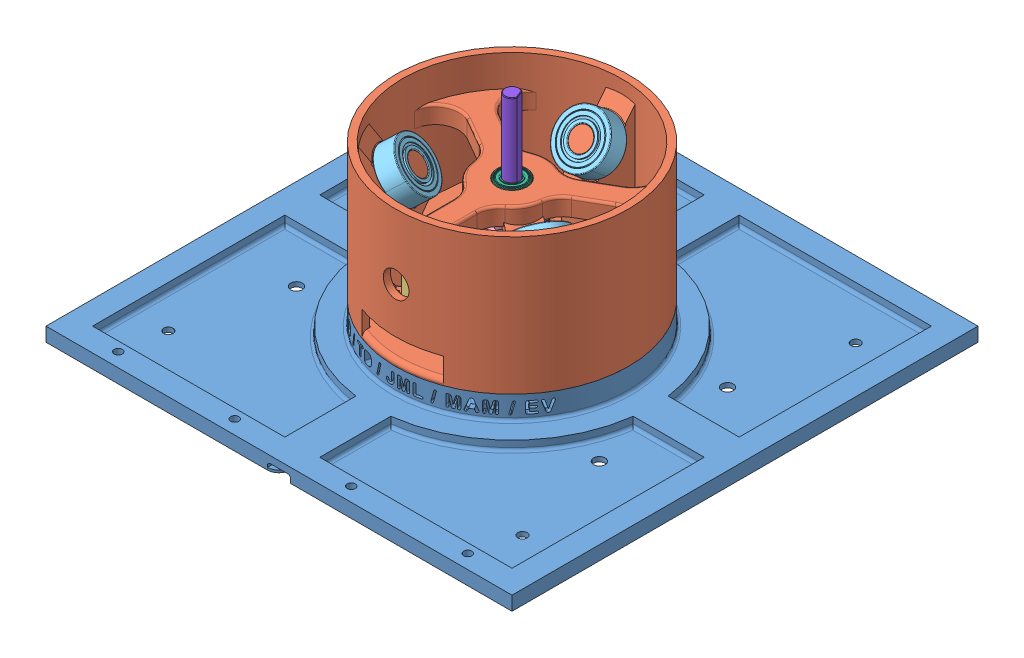
SolidWorks assembly Socle, configuration Défaut. Lengths in mm.
Overall size (200 92.98 200).
27 component instances, 14 part files, 141 mates.
Components (placement in the parent):
- robot_base_plate-2: robot_base_plate [Défaut] at (0 -6 0) size (200 16 200)
- Support_Bearing_V4-1: Support_Bearing_V4 [Défaut] at (0 10 0) x (0 0 1) z (-1 0 0) size (100 58.5 100)
- XL430-W250-1: XL430-W250 [Défaut] at (0 36 0) x (-1 0 0) z (0 1 0) size (28.5 46.5 36.18)
- Coupler_Joint1-1: Coupler_Joint1 [Défaut] at (0 36 0) x (0.374118 0 0.927381) z (-0.927381 0 0.374118) size (22.5 6 20.75)
- bearing-1: bearing [Default] at (0 52.1597 -32.8363) x (0.617014 0.614506 -0.491605) z (0 -0.624695 -0.780869) size (22.23 22.23 8.73)
- bearing-2: bearing [Default] at (-28.437 52.1597 16.4181) x (0.592905 -0.776094 -0.214808) z (-0.676252 -0.624695 0.390434) size (22.23 22.23 8.73)
- bearing-3: bearing [Default] at (28.437 52.1597 16.4181) x (0.541002 0.780869 0.312348) z (0.676252 -0.624695 0.390434) size (22.23 22.23 8.73)
- 535198-1: 535198 [Default] at (0 55.6322 0) x (-0.798975 0 -0.601364) z (-0.601364 0 0.798975) size (13.87 4.75 13.87)
- 6432K12-1: 6432K12 [Défaut] at (0 43.2374 0) x (-0.932842 0 -0.360287) z (0.360287 0 -0.932842) size (12.48 7.15 12.48)
- shaft-1: shaft [2po] at (0 61.5779 0) x (0.374118 0 0.927381) z (0 1 0) size (6.35 5.71 50.8)
- M3-8mm_91292A112_TYPE 18-8 SS SOCKET HEAD CAP SCREW-1: M3-8mm_91292A112_TYPE 18-8 SS SOCKET HEAD CAP SCREW [91292A112] at (2.3555 39 -0.9503) x (0.050445 0.990868 0.125045) z (-0.927381 0 0.374118) size (5.5 5.5 11.2)
- M3-NUT_90710A030_TYPE 18-8 SS THIN HEX NUT - DIN 439B-9: M3-NUT_90710A030_TYPE 18-8 SS THIN HEX NUT - DIN 439B [90710A030] at (5.3324 39 -2.1512) x (0.332828 -0.456677 0.825028) z (0.170851 0.889632 0.423514) size (5.5 2.19 6.35)
- M2-16mm_91292A002_TYPE 18-8 SS SOCKET HEAD CAP SCREW-1: M2-16mm_91292A002_TYPE 18-8 SS SOCKET HEAD CAP SCREW [91292A002] at (-11 13.5 32) x (0.96925 0 -0.246077) z (0 1 0) size (3.8 3.8 18.16)
- M2-16mm_91292A002_TYPE 18-8 SS SOCKET HEAD CAP SCREW-2: M2-16mm_91292A002_TYPE 18-8 SS SOCKET HEAD CAP SCREW [91292A002] at (11 13.5 32) x (0.905509 0 -0.424327) z (0 1 0) size (3.8 3.8 18.16)
- M2-16mm_91292A002_TYPE 18-8 SS SOCKET HEAD CAP SCREW-3: M2-16mm_91292A002_TYPE 18-8 SS SOCKET HEAD CAP SCREW [91292A002] at (-11 13.5 -8) x (0.792745 0 -0.609554) z (0 1 0) size (3.8 3.8 18.16)
- M2-16mm_91292A002_TYPE 18-8 SS SOCKET HEAD CAP SCREW-4: M2-16mm_91292A002_TYPE 18-8 SS SOCKET HEAD CAP SCREW [91292A002] at (11 13.5 -8) x (0.627754 0 -0.778412) z (0 1 0) size (3.8 3.8 18.16)
- M4-NUT_90710A035_TYPE 18-8 SS THIN HEX NUT - DIN 439B-10: M4-NUT_90710A035_TYPE 18-8 SS THIN HEX NUT - DIN 439B [90710A035] at (-22.5 13.6 30) size (7 2.75 8.08)
- M4-20mm_91292A118_TYPE 18-8 SS SOCKET HEAD CAP SCREW-7: M4-20mm_91292A118_TYPE 18-8 SS SOCKET HEAD CAP SCREW [91292A118] at (-22.5 19 30) x (0.815208 0 -0.579168) z (0 1 0) size (7 7 24.38)
- M4-20mm_91292A118_TYPE 18-8 SS SOCKET HEAD CAP SCREW-8: M4-20mm_91292A118_TYPE 18-8 SS SOCKET HEAD CAP SCREW [91292A118] at (22.5 19 30) x (-0.815208 0 -0.579168) z (0 1 0) size (7 7 24.38)
- M4-NUT_90710A035_TYPE 18-8 SS THIN HEX NUT - DIN 439B-11: M4-NUT_90710A035_TYPE 18-8 SS THIN HEX NUT - DIN 439B [90710A035] at (22.5 13.6 30) x (-1 0 0) z (0 0 -1) size (7 2.75 8.08)
- M4-20mm_91292A118_TYPE 18-8 SS SOCKET HEAD CAP SCREW-9: M4-20mm_91292A118_TYPE 18-8 SS SOCKET HEAD CAP SCREW [91292A118] at (-22.5 19 -30) x (0.815208 0 0.579168) z (0 1 0) size (7 7 24.38)
- M4-NUT_90710A035_TYPE 18-8 SS THIN HEX NUT - DIN 439B-12: M4-NUT_90710A035_TYPE 18-8 SS THIN HEX NUT - DIN 439B [90710A035] at (-22.5 13.6 -30) size (7 2.75 8.08)
- M4-20mm_91292A118_TYPE 18-8 SS SOCKET HEAD CAP SCREW-10: M4-20mm_91292A118_TYPE 18-8 SS SOCKET HEAD CAP SCREW [91292A118] at (22.5 19 -30) x (-0.815208 0 0.579168) z (0 1 0) size (7 7 24.38)
- M4-NUT_90710A035_TYPE 18-8 SS THIN HEX NUT - DIN 439B-13: M4-NUT_90710A035_TYPE 18-8 SS THIN HEX NUT - DIN 439B [90710A035] at (22.5 13.6 -30) x (-1 0 0) z (0 0 -1) size (7 2.75 8.08)
- M2-4mm_TYPE 18-8 SS SOCKET HEAD CAP SCREW-1: M2-4mm_TYPE 18-8 SS SOCKET HEAD CAP SCREW [91292A832] at (2.9929 34 7.419) x (0.957551 0 -0.288264) z (0 -1 0) size (3.8 3.8 6.09)
- M2-4mm_TYPE 18-8 SS SOCKET HEAD CAP SCREW-2: M2-4mm_TYPE 18-8 SS SOCKET HEAD CAP SCREW [91292A832] at (-2.9929 34 -7.419) x (0.170389 0 -0.985377) z (0 -1 0) size (3.8 3.8 6.09)
- M2-4mm_TYPE 18-8 SS SOCKET HEAD CAP SCREW-3: M2-4mm_TYPE 18-8 SS SOCKET HEAD CAP SCREW [91292A832] at (-7.419 34 2.9929) x (0.981537 0 0.191272) z (0 -1 0) size (3.8 3.8 6.09)
Mates (geometry in assembly coordinates):
- Coïncidente4: coincident aligned: plane of XL430-W250-1 through (0 36 0) normal (0 0 1)
- Coïncidente5: coincident anti-aligned: plane of XL430-W250-1 through (0 36 0) normal (-1 0 0)
- Coïncidente6: coincident anti-aligned: plane of XL430-W250-1 through (0 0 0) normal (0 -1 0)
- Coïncidente7: coincident anti-aligned: plane of Rpi3Bplus-1 through (39.75 0 197.5) normal (0 -1 0)
- Coïncidente8: coincident anti-aligned: plane of OpenCR-1 through (-20.75 0 217.25) normal (0 -1 0)
- Parallèle2: parallel aligned: plane of Support_Bearing_V4-1 through (0 12.5 0) normal (0 1 0)
- Coïncidente13: coincident anti-aligned: plane of Support_Bearing_V4-1 through (0 10 0) normal (-1 0 0)
- Coïncidente14: coincident aligned: plane of Support_Bearing_V4-1 through (0 10 0) normal (0 0 1)
- Coaxiale7: concentric anti-aligned: cylinder of bearing-1 through (0 49.1594 -36.5867) axis (0 0.624695 0.780869) radius 4.7625; cylinder of Support_Bearing_V4-1 through (0 54.7421 -29.6083) axis (0 -0.624695 -0.780869) radius 4.6875
- Coïncidente15: coincident anti-aligned: plane of bearing-1 through (0 49.4322 -36.2457) normal (0 -0.624695 -0.780869); plane of Support_Bearing_V4-1 through (-6.25 63.5 -47.5) normal (0 0.624695 0.780869)
- Distance2: distance = 10 mm aligned: plane of XL430-W250-1 through (0 0 0) normal (0 -1 0); plane of Support_Bearing_V4-1 through (0 10 0) normal (0 -1 0)
- Coaxiale8: concentric anti-aligned: cylinder of Support_Bearing_V4-1 through (-25.6416 54.7421 14.8042) axis (-0.676252 -0.624695 0.390434) radius 4.6875; cylinder of bearing-2 through (-31.685 49.1594 18.2933) axis (0.676252 0.624695 -0.390434) radius 4.7625
- Coaxiale9: concentric anti-aligned: cylinder of Support_Bearing_V4-1 through (25.6416 54.7421 14.8042) axis (0.676252 -0.624695 0.390434) radius 4.6875; cylinder of bearing-3 through (31.685 49.1594 18.2933) axis (-0.676252 0.624695 -0.390434) radius 4.7625
- Coïncidente16: coincident anti-aligned: plane of Support_Bearing_V4-1 through (44.2612 63.5 18.3373) normal (-0.676252 0.624695 -0.390434); plane of bearing-3 through (31.3897 49.4322 18.1229) normal (0.676252 -0.624695 0.390434)
- Coïncidente17: coincident anti-aligned: plane of Support_Bearing_V4-1 through (-38.0112 63.5 29.1627) normal (0.676252 0.624695 -0.390434); plane of bearing-2 through (-31.3897 49.4322 18.1229) normal (-0.676252 -0.624695 0.390434)
- Coïncidente18: coincident aligned: plane of robot_base_plate-2 through (0 0 0) normal (0 1 0)
- Coïncidente19: coincident aligned: plane of robot_base_plate-2 through (0 -6 0) normal (1 0 0)
- Coïncidente20: coincident aligned: plane of robot_base_plate-2 through (0 -6 0) normal (0 0 1)
- Coaxiale10: concentric aligned: cylinder of OpenCR-1 through (-89.25 1.7 118.75) axis (0 -1 0) radius 2; cylinder of Base_Controler-1 through (-89.25 2.95 118.75) axis (0 -1 0) radius 1.75
- Coaxiale11: concentric aligned: cylinder of OpenCR-1 through (-23.25 1.7 214.75) axis (0 -1 0) radius 2; cylinder of Base_Controler-1 through (-23.25 2.95 214.75) axis (0 -1 0) radius 1.75
- Coaxiale12: concentric aligned: cylinder of Rpi3Bplus-1 through (89.25 1.4986 119) axis (0 -1 0) radius 1.375; cylinder of Base_Controler-1 through (89.25 2.95 119) axis (0 -1 0) radius 1.15
- Coaxiale13: concentric aligned: cylinder of Rpi3Bplus-1 through (89.25 1.4986 177) axis (0 -1 0) radius 1.375; cylinder of Base_Controler-1 through (89.25 2.95 177) axis (0 -1 0) radius 1.15
- Coïncidente24: coincident aligned: plane of robot_base_plate-2 through (100 -4 100) normal (1 0 0); plane of Base_Controler-1 through (100 33.95 225.5) normal (1 0 0)
- Coïncidente26: coincident: line of robot_base_plate-2 through (-100 0 100) axis (1 0 0); plane of Base_Controler-1 through (-100 33.95 100) normal (0 0 -1)
- Coïncidente27: coincident anti-aligned: plane of Cover_Controler-1 through (-11.6809 33.95 140.7407) normal (0 -1 0); plane of Base_Controler-1 through (-100 33.95 225.5) normal (0 1 0)
- Largeur1: width anti-aligned: plane of Cover_Controler-1 through (96.75 28.95 222.25) normal (0 0 1); plane of Base_Controler-1 through (-96.75 28.95 103.25) normal (0 0 -1); plane of Cover_Controler-1 through (-97 -3.05 222.5) normal (0 0 -1); plane of Base_Controler-1 through (-97 -3.05 103) normal (0 0 1)
- Largeur2: width anti-aligned: plane of Cover_Controler-1 through (-96.75 28.95 222.25) normal (-1 0 0); plane of Cover_Controler-1 through (96.75 28.95 103.25) normal (1 0 0); plane of Base_Controler-1 through (-97 -3.05 103) normal (1 0 0); plane of Base_Controler-1 through (97 -3.05 103) normal (-1 0 0)
- Coaxiale17: concentric aligned: cylinder of XL430-W250-1 through (0 38.35 0) axis (0 -1 0) radius 9.75; cylinder of 535198-1 through (0 55.6322 0) axis (0 -1 0) radius 3.175
- Coaxiale18: concentric aligned: cylinder of XL430-W250-1 through (0 38.35 0) axis (0 -1 0) radius 9.75; cylinder of 6432K12-1 through (0 50.3824 0) axis (0 -1 0) radius 3.175
- Distance3: distance = 0.5 mm anti-aligned: plane of 535198-1 through (0 50.8824 0) normal (0 -1 0); plane of 6432K12-1 through (0 50.3824 0) normal (0 1 0)
- Coaxiale19: concentric aligned: cylinder of XL430-W250-1 through (0 38.35 0) axis (0 -1 0) radius 9.75; cylinder of shaft-1 through (0 86.9779 0) axis (0 -1 0) radius 3.175
- Coïncidente29: coincident anti-aligned: plane of XL430-W250-1 through (5 36.1779 4.5585) normal (0 1 0); plane of shaft-1 through (0 36.1779 0) normal (0 -1 0)
- Coïncidente31: coincident anti-aligned: plane of 535198-1 through (0 52 0) normal (0 1 0); plane of Support_Bearing_V4-1 through (0 52 0) normal (0 -1 0)
- Coaxiale21: concentric aligned: cylinder of shaft-1 through (0 86.9779 0) axis (0 -1 0) radius 3.175; circle of ?
- Parallèle4: parallel anti-aligned: plane of shaft-1 through (3.0682 86.9779 0.8164) normal (0.927381 0 -0.374118); plane of ? through (1.5332 91 4.093) normal (0.454214 0 -0.890893)
- Coïncidente32: coincident: plane of ? through (29.3995 63.5 14.9891) normal (0.890893 0 0.454214); plane of ? through (29.3995 263.25 14.9891) normal (-0.890893 0 -0.454214)
- Coaxiale22: concentric: cylinder of ? through (11.544 271.25 18.2328) axis (-0.890893 0 -0.454214) radius 1.35; cylinder of ? through (24.4031 271.25 24.7889) axis (-0.890893 0 -0.454214) radius 1.3
- Coaxiale23: concentric: cylinder of ? through (21.5367 231.25 -1.3669) axis (-0.890893 0 -0.454214) radius 1.35; cylinder of ? through (34.3958 231.25 5.1892) axis (-0.890893 0 -0.454214) radius 1.3
- Coaxiale24: concentric: cylinder of ? through (-40.982 263.25 -20.8943) axis (0.890893 0 0.454214) radius 3.25; cylinder of ? through (-20.8899 263.25 -10.6505) axis (0.890893 0 0.454214) radius 3.175
- Coïncidente33: coincident: plane of ? through (-17.654 263.25 -9.0007) normal (0.890893 0 0.454214); plane of ? through (-17.654 263.25 -9.0007) normal (-0.890893 0 -0.454214)
- Parallèle6: parallel anti-aligned: plane of Support_Bearing_V4-1 through (3.125 10 -5.4127) normal (0.5 0 -0.866025); plane of bearing-3 through (28.437 52.1597 16.4181) normal (-0.5 0 0.866025)
- Coïncidente34: coincident aligned: plane of Support_Bearing_V4-1 through (0 68.5 0) normal (0 1 0); plane of ? through (0 68.5 0) normal (0 1 0)
- Coaxiale25: concentric: cylinder of ? through (29.3995 263.25 14.9891) axis (0.890893 0 0.454214) radius 11.25; cylinder of ? through (22.2723 263.25 11.3553) axis (0.890893 0 0.454214) radius 11
- Coïncidente35: coincident: plane of ? through (27.6177 263.25 14.0806) normal (-0.890893 0 -0.454214); plane of ? through (27.6177 263.25 14.0806) normal (0.890893 0 0.454214)
- Coaxiale26: concentric: cylinder of ? through (-40.982 263.25 -20.8943) axis (0.890893 0 0.454214) radius 6.5; cylinder of ? through (20.8898 263.25 10.6505) axis (-0.890893 0 -0.454214) radius 3.175
- Coïncidente37: coincident: plane of ? through (17.6539 263.25 9.0007) normal (-0.890893 0 -0.454214); plane of ? through (17.6539 263.25 9.0007) normal (0.890893 0 0.454214)
- Coïncidente38: coincident anti-aligned: plane of robot_base_plate-2 through (0 0 0) normal (0 1 0); plane of Base_Controler-1 through (100 0 90) normal (0 -1 0)
- Coaxiale27: concentric anti-aligned: cylinder of Cover_Controler-1 through (-71.75 35.95 178.75) axis (0 1 0) radius 1.95; cylinder of 40x40x10 DC Fan-1 through (-71.75 23.45 178.75) axis (0 -1 0) radius 1.725
- Coaxiale28: concentric anti-aligned: cylinder of Cover_Controler-1 through (-39.75 35.95 146.75) axis (0 1 0) radius 1.95; cylinder of 40x40x10 DC Fan-1 through (-39.75 23.45 146.75) axis (0 -1 0) radius 1.725
- Coïncidente39: coincident anti-aligned: plane of Cover_Controler-1 through (-11.6809 33.95 140.7407) normal (0 -1 0); plane of 40x40x10 DC Fan-1 through (-71.75 33.95 146.75) normal (0 1 0)
- Coaxiale29: concentric anti-aligned: cylinder of Cover_Controler-1 through (39.75 35.95 178.75) axis (0 1 0) radius 1.95; cylinder of 40x40x10 DC Fan-2 through (39.75 23.45 178.75) axis (0 -1 0) radius 1.725
- Coaxiale30: concentric anti-aligned: cylinder of Cover_Controler-1 through (71.75 35.95 146.75) axis (0 1 0) radius 1.95; cylinder of 40x40x10 DC Fan-2 through (71.75 23.45 146.75) axis (0 -1 0) radius 1.725
- Coïncidente40: coincident anti-aligned: plane of Cover_Controler-1 through (-11.6809 33.95 140.7407) normal (0 -1 0); plane of 40x40x10 DC Fan-2 through (39.75 33.95 146.75) normal (0 1 0)
- Coaxiale31: concentric anti-aligned: cylinder of Base_Controler-1 through (75 -6.05 94) axis (0 1 0) radius 2.2; cylinder of M4-8mm_91292A108_TYPE 18-8 SS SOCKET HEAD CAP SCREW-1 through (75 7 94) axis (0 -1 0) radius 3.5
- Coïncidente41: coincident anti-aligned: plane of Base_Controler-1 through (100 3 90) normal (0 1 0); plane of M4-8mm_91292A108_TYPE 18-8 SS SOCKET HEAD CAP SCREW-1 through (75 3 94) normal (0 -1 0)
- Coaxiale32: concentric anti-aligned: cylinder of Base_Controler-1 through (25 -6.05 94) axis (0 1 0) radius 2.2; cylinder of M4-8mm_91292A108_TYPE 18-8 SS SOCKET HEAD CAP SCREW-2 through (25 7 94) axis (0 -1 0) radius 3.5
- Coïncidente42: coincident anti-aligned: plane of Base_Controler-1 through (100 3 90) normal (0 1 0); plane of M4-8mm_91292A108_TYPE 18-8 SS SOCKET HEAD CAP SCREW-2 through (25 3 94) normal (0 -1 0)
- Coaxiale33: concentric anti-aligned: cylinder of Base_Controler-1 through (-25 -6.05 94) axis (0 1 0) radius 2.2; cylinder of M4-8mm_91292A108_TYPE 18-8 SS SOCKET HEAD CAP SCREW-4 through (-25 7 94) axis (0 -1 0) radius 3.5
- Coïncidente43: coincident anti-aligned: plane of Base_Controler-1 through (100 3 90) normal (0 1 0); plane of M4-8mm_91292A108_TYPE 18-8 SS SOCKET HEAD CAP SCREW-4 through (-25 3 94) normal (0 -1 0)
- Coaxiale34: concentric anti-aligned: cylinder of Base_Controler-1 through (-75 -6.05 94) axis (0 1 0) radius 2.2; cylinder of M4-8mm_91292A108_TYPE 18-8 SS SOCKET HEAD CAP SCREW-6 through (-75 7 94) axis (0 -1 0) radius 3.5
- Coïncidente44: coincident anti-aligned: plane of Base_Controler-1 through (100 3 90) normal (0 1 0); plane of M4-8mm_91292A108_TYPE 18-8 SS SOCKET HEAD CAP SCREW-6 through (-75 3 94) normal (0 -1 0)
- Coaxiale35: concentric anti-aligned: cylinder of robot_base_plate-2 through (22.5 -6 -30) axis (0 -1 0) radius 4; cylinder of M5-20mm_TYPE 18-8 SS SOCKET HEAD CAP SCREW-1 through (22.5 -5 -30) axis (0 1 0) radius 4.5
- Coïncidente45: coincident anti-aligned: plane of robot_base_plate-2 through (24.75 -1 -30) normal (0 -1 0); plane of M5-20mm_TYPE 18-8 SS SOCKET HEAD CAP SCREW-1 through (22.5 -1 -30) normal (0 1 0)
- Coaxiale36: concentric anti-aligned: cylinder of robot_base_plate-2 through (22.5 -6 30) axis (0 -1 0) radius 4; cylinder of M5-20mm_TYPE 18-8 SS SOCKET HEAD CAP SCREW-2 through (22.5 -5 30) axis (0 1 0) radius 4.5
- Coïncidente46: coincident anti-aligned: plane of robot_base_plate-2 through (24.75 -1 30) normal (0 -1 0); plane of M5-20mm_TYPE 18-8 SS SOCKET HEAD CAP SCREW-2 through (22.5 -1 30) normal (0 1 0)
- Coaxiale37: concentric anti-aligned: cylinder of robot_base_plate-2 through (-22.5 -6 -30) axis (0 -1 0) radius 4; cylinder of M5-20mm_TYPE 18-8 SS SOCKET HEAD CAP SCREW-4 through (-22.5 -5 -30) axis (0 1 0) radius 4.5
- Coïncidente47: coincident anti-aligned: plane of robot_base_plate-2 through (-20.25 -1 -30) normal (0 -1 0); plane of M5-20mm_TYPE 18-8 SS SOCKET HEAD CAP SCREW-4 through (-22.5 -1 -30) normal (0 1 0)
- Coaxiale38: concentric anti-aligned: cylinder of robot_base_plate-2 through (-22.5 -6 30) axis (0 -1 0) radius 4; cylinder of M5-20mm_TYPE 18-8 SS SOCKET HEAD CAP SCREW-6 through (-22.5 -5 30) axis (0 1 0) radius 4.5
- Coïncidente48: coincident anti-aligned: plane of robot_base_plate-2 through (-20.25 -1 30) normal (0 -1 0); plane of M5-20mm_TYPE 18-8 SS SOCKET HEAD CAP SCREW-6 through (-22.5 -1 30) normal (0 1 0)
- Coaxiale39: concentric aligned: circle of Support_Bearing_V4-1; circle of M4-NUT_90710A035_TYPE 18-8 SS THIN HEX NUT - DIN 439B-1
- Parallèle7: parallel anti-aligned: plane of Support_Bearing_V4-1 through (19 15 -27.9793) normal (0.5 0 -0.866025); plane of M5-NUT_TYPE 18-8 SS THIN HEX NUT - DIN 439B-1 through (18.5 15.5 -27.6906) normal (-0.5 0 0.866025)
- Coïncidente49: coincident anti-aligned: plane of Support_Bearing_V4-1 through (0 12.5 0) normal (0 1 0); plane of M5-NUT_TYPE 18-8 SS THIN HEX NUT - DIN 439B-1 through (18.5 12.5 -32.3094) normal (0 -1 0)
- Coaxiale41: concentric aligned: cylinder of Support_Bearing_V4-1 through (-22.5 9.999 -30) axis (0 1 0) radius 2.25; unknown of M4-NUT_90710A035_TYPE 18-8 SS THIN HEX NUT - DIN 439B-3
- Parallèle9: parallel anti-aligned: plane of Support_Bearing_V4-1 through (-26 15 -27.9793) normal (1 0 0); plane of M5-NUT_TYPE 18-8 SS THIN HEX NUT - DIN 439B-3 through (-26.5 15.5 -32.3094) normal (-1 0 0)
- Coïncidente52: coincident anti-aligned: plane of Support_Bearing_V4-1 through (0 12.5 0) normal (0 1 0); plane of M5-NUT_TYPE 18-8 SS THIN HEX NUT - DIN 439B-3 through (-22.5 12.5 -34.6188) normal (0 -1 0)
- Coïncidente53: coincident anti-aligned: plane of Support_Bearing_V4-1 through (0 12.5 0) normal (0 1 0); plane of M5-NUT_TYPE 18-8 SS THIN HEX NUT - DIN 439B-4 through (-22.5 12.5 25.3812) normal (0 -1 0)
- Coaxiale42: concentric aligned: unknown of Support_Bearing_V4-1; unknown of M4-NUT_90710A035_TYPE 18-8 SS THIN HEX NUT - DIN 439B-4
- Parallèle10: parallel anti-aligned: plane of Support_Bearing_V4-1 through (-26 15 27.9793) normal (1 0 0); plane of M5-NUT_TYPE 18-8 SS THIN HEX NUT - DIN 439B-4 through (-26.5 15.5 27.6906) normal (-1 0 0)
- Coïncidente54: coincident anti-aligned: plane of Support_Bearing_V4-1 through (0 12.5 0) normal (0 1 0); plane of M5-NUT_TYPE 18-8 SS THIN HEX NUT - DIN 439B-5 through (22.5 12.5 25.3812) normal (0 -1 0)
- Coaxiale43: concentric aligned: unknown of Support_Bearing_V4-1; unknown of M4-NUT_90710A035_TYPE 18-8 SS THIN HEX NUT - DIN 439B-5
- Parallèle11: parallel anti-aligned: plane of Support_Bearing_V4-1 through (19 15 32.0207) normal (1 0 0); plane of M5-NUT_TYPE 18-8 SS THIN HEX NUT - DIN 439B-5 through (18.5 15.5 27.6906) normal (-1 0 0)
- Coaxiale44: concentric anti-aligned: cylinder of Cover_Controler-1 through (-71.75 35.95 178.75) axis (0 1 0) radius 1.95; cylinder of M3-16mm_91292A115_TYPE 18-8 SS SOCKET HEAD CAP SCREW-1 through (-71.75 38.95 178.75) axis (0 -1 0) radius 2.75
- Coïncidente55: coincident anti-aligned: plane of Cover_Controler-1 through (-11.6809 35.95 140.7407) normal (0 1 0); plane of M3-16mm_91292A115_TYPE 18-8 SS SOCKET HEAD CAP SCREW-1 through (-71.75 35.95 178.75) normal (0 -1 0)
- Coïncidente56: coincident anti-aligned: plane of Cover_Controler-1 through (-11.6809 35.95 140.7407) normal (0 1 0); plane of M3-16mm_91292A115_TYPE 18-8 SS SOCKET HEAD CAP SCREW-2 through (-39.75 35.95 178.75) normal (0 -1 0)
- Coaxiale45: concentric anti-aligned: cylinder of Cover_Controler-1 through (-39.75 35.95 178.75) axis (0 1 0) radius 1.95; cylinder of M3-16mm_91292A115_TYPE 18-8 SS SOCKET HEAD CAP SCREW-2 through (-39.75 38.95 178.75) axis (0 -1 0) radius 2.75
- Coïncidente57: coincident anti-aligned: plane of Cover_Controler-1 through (-11.6809 35.95 140.7407) normal (0 1 0); plane of M3-16mm_91292A115_TYPE 18-8 SS SOCKET HEAD CAP SCREW-3 through (-39.75 35.95 146.75) normal (0 -1 0)
- Coaxiale46: concentric anti-aligned: cylinder of Cover_Controler-1 through (-39.75 35.95 146.75) axis (0 1 0) radius 1.95; cylinder of M3-16mm_91292A115_TYPE 18-8 SS SOCKET HEAD CAP SCREW-3 through (-39.75 38.95 146.75) axis (0 -1 0) radius 2.75
- Coïncidente58: coincident anti-aligned: plane of Cover_Controler-1 through (-11.6809 35.95 140.7407) normal (0 1 0); plane of M3-16mm_91292A115_TYPE 18-8 SS SOCKET HEAD CAP SCREW-4 through (-71.75 35.95 146.75) normal (0 -1 0)
- Coaxiale47: concentric anti-aligned: cylinder of Cover_Controler-1 through (-71.75 35.95 146.75) axis (0 1 0) radius 1.95; cylinder of M3-16mm_91292A115_TYPE 18-8 SS SOCKET HEAD CAP SCREW-4 through (-71.75 38.95 146.75) axis (0 -1 0) radius 2.75
- Coïncidente60: coincident anti-aligned: plane of Cover_Controler-1 through (-11.6809 35.95 140.7407) normal (0 1 0); plane of M3-16mm_91292A115_TYPE 18-8 SS SOCKET HEAD CAP SCREW-6 through (71.75 35.95 178.75) normal (0 -1 0)
- Coaxiale49: concentric anti-aligned: cylinder of Cover_Controler-1 through (71.75 35.95 178.75) axis (0 1 0) radius 1.95; cylinder of M3-16mm_91292A115_TYPE 18-8 SS SOCKET HEAD CAP SCREW-6 through (71.75 38.95 178.75) axis (0 -1 0) radius 2.75
- Coïncidente61: coincident anti-aligned: plane of Cover_Controler-1 through (-11.6809 35.95 140.7407) normal (0 1 0); plane of M3-16mm_91292A115_TYPE 18-8 SS SOCKET HEAD CAP SCREW-7 through (71.75 35.95 146.75) normal (0 -1 0)
- Coaxiale50: concentric anti-aligned: cylinder of Cover_Controler-1 through (71.75 35.95 146.75) axis (0 1 0) radius 1.95; cylinder of M3-16mm_91292A115_TYPE 18-8 SS SOCKET HEAD CAP SCREW-7 through (71.75 38.95 146.75) axis (0 -1 0) radius 2.75
- Coïncidente62: coincident anti-aligned: plane of Cover_Controler-1 through (-11.6809 35.95 140.7407) normal (0 1 0); plane of M3-16mm_91292A115_TYPE 18-8 SS SOCKET HEAD CAP SCREW-8 through (39.75 35.95 146.75) normal (0 -1 0)
- Coaxiale51: concentric anti-aligned: cylinder of Cover_Controler-1 through (39.75 35.95 146.75) axis (0 1 0) radius 1.95; cylinder of M3-16mm_91292A115_TYPE 18-8 SS SOCKET HEAD CAP SCREW-8 through (39.75 38.95 146.75) axis (0 -1 0) radius 2.75
- Coïncidente64: coincident anti-aligned: plane of Cover_Controler-1 through (-11.6809 35.95 140.7407) normal (0 1 0); plane of M3-16mm_91292A115_TYPE 18-8 SS SOCKET HEAD CAP SCREW-11 through (39.75 35.95 178.75) normal (0 -1 0)
- Coaxiale53: concentric anti-aligned: cylinder of Cover_Controler-1 through (39.75 35.95 178.75) axis (0 1 0) radius 1.95; cylinder of M3-16mm_91292A115_TYPE 18-8 SS SOCKET HEAD CAP SCREW-11 through (39.75 38.95 178.75) axis (0 -1 0) radius 2.75
- Coïncidente66: coincident anti-aligned: plane of 40x40x10 DC Fan-2 through (55.75 23.45 162.75) normal (0 -1 0); plane of M3-NUT_90710A030_TYPE 18-8 SS THIN HEX NUT - DIN 439B-1 through (69 23.45 177.1623) normal (0 1 0)
- Coaxiale54: concentric anti-aligned: circle of 40x40x10 DC Fan-2; circle of M3-NUT_90710A030_TYPE 18-8 SS THIN HEX NUT - DIN 439B-1
- Coïncidente67: coincident anti-aligned: plane of 40x40x10 DC Fan-2 through (55.75 23.45 162.75) normal (0 -1 0); plane of M3-NUT_90710A030_TYPE 18-8 SS THIN HEX NUT - DIN 439B-2 through (68.7501 23.45 145.709) normal (0 1 0)
- Coaxiale55: concentric anti-aligned: unknown of 40x40x10 DC Fan-2; unknown of M3-NUT_90710A030_TYPE 18-8 SS THIN HEX NUT - DIN 439B-2
- Coïncidente68: coincident anti-aligned: plane of 40x40x10 DC Fan-2 through (55.75 23.45 162.75) normal (0 -1 0); plane of M3-NUT_90710A030_TYPE 18-8 SS THIN HEX NUT - DIN 439B-3 through (36.5962 23.45 146.3802) normal (0 1 0)
- Coaxiale56: concentric anti-aligned: unknown of 40x40x10 DC Fan-2; unknown of M3-NUT_90710A030_TYPE 18-8 SS THIN HEX NUT - DIN 439B-3
- Coïncidente69: coincident anti-aligned: plane of 40x40x10 DC Fan-2 through (55.75 23.45 162.75) normal (0 -1 0); plane of M3-NUT_90710A030_TYPE 18-8 SS THIN HEX NUT - DIN 439B-4 through (36.5974 23.45 179.1298) normal (0 1 0)
- Coaxiale57: concentric anti-aligned: unknown of 40x40x10 DC Fan-2; unknown of M3-NUT_90710A030_TYPE 18-8 SS THIN HEX NUT - DIN 439B-4
- Coïncidente70: coincident anti-aligned: plane of 40x40x10 DC Fan-2 through (55.75 23.45 162.75) normal (0 -1 0); plane of M3-NUT_90710A030_TYPE 18-8 SS THIN HEX NUT - DIN 439B-5 through (-42.7207 23.45 179.8717) normal (0 1 0)
- Coaxiale58: concentric anti-aligned: unknown of 40x40x10 DC Fan-1; unknown of M3-NUT_90710A030_TYPE 18-8 SS THIN HEX NUT - DIN 439B-5
- Coïncidente71: coincident anti-aligned: plane of 40x40x10 DC Fan-2 through (55.75 23.45 162.75) normal (0 -1 0); plane of M3-NUT_90710A030_TYPE 18-8 SS THIN HEX NUT - DIN 439B-6 through (-74.3929 23.45 180.5102) normal (0 1 0)
- Coaxiale59: concentric anti-aligned: unknown of 40x40x10 DC Fan-1; unknown of M3-NUT_90710A030_TYPE 18-8 SS THIN HEX NUT - DIN 439B-6
- Coïncidente72: coincident anti-aligned: plane of 40x40x10 DC Fan-2 through (55.75 23.45 162.75) normal (0 -1 0); plane of M3-NUT_90710A030_TYPE 18-8 SS THIN HEX NUT - DIN 439B-7 through (-74.0056 23.45 148.9851) normal (0 1 0)
- Coaxiale60: concentric anti-aligned: unknown of 40x40x10 DC Fan-1; unknown of M3-NUT_90710A030_TYPE 18-8 SS THIN HEX NUT - DIN 439B-7
- Coïncidente73: coincident anti-aligned: plane of 40x40x10 DC Fan-2 through (55.75 23.45 162.75) normal (0 -1 0); plane of M3-NUT_90710A030_TYPE 18-8 SS THIN HEX NUT - DIN 439B-8 through (-41.6567 23.45 149.2893) normal (0 1 0)
- Coaxiale61: concentric anti-aligned: unknown of 40x40x10 DC Fan-1; unknown of M3-NUT_90710A030_TYPE 18-8 SS THIN HEX NUT - DIN 439B-8
- Coïncidente74: coincident anti-aligned: plane of shaft-1 through (3.0682 86.9779 0.8164) normal (0.927381 0 -0.374118); plane of M3-8mm_91292A112_TYPE 18-8 SS SOCKET HEAD CAP SCREW-1 through (2.3555 39 -0.9503) normal (-0.927381 0 0.374118)
- Coaxiale63: concentric anti-aligned: cylinder of M3-8mm_91292A112_TYPE 18-8 SS SOCKET HEAD CAP SCREW-1 through (12.5567 39 -5.0656) axis (-0.927381 0 0.374118) radius 2.75; circle of M3-NUT_90710A030_TYPE 18-8 SS THIN HEX NUT - DIN 439B-9
- Coaxiale64: concentric anti-aligned: cylinder of robot_base_plate-2 through (-11 -6 32) axis (0 -1 0) radius 2.2; cylinder of M2-16mm_91292A002_TYPE 18-8 SS SOCKET HEAD CAP SCREW-1 through (-11 -4.5 32) axis (0 1 0) radius 1.9
- Coïncidente76: coincident anti-aligned: plane of robot_base_plate-2 through (-9.8 -2.5 32) normal (0 -1 0); plane of M2-16mm_91292A002_TYPE 18-8 SS SOCKET HEAD CAP SCREW-1 through (-11 -2.5 32) normal (0 1 0)
- Coïncidente77: coincident anti-aligned: plane of robot_base_plate-2 through (-9.8 -2.5 32) normal (0 -1 0); plane of M2-16mm_91292A002_TYPE 18-8 SS SOCKET HEAD CAP SCREW-2 through (11 -2.5 32) normal (0 1 0)
- Coaxiale65: concentric anti-aligned: cylinder of robot_base_plate-2 through (11 -6 32) axis (0 -1 0) radius 2.2; cylinder of M2-16mm_91292A002_TYPE 18-8 SS SOCKET HEAD CAP SCREW-2 through (11 -4.5 32) axis (0 1 0) radius 1.9
- Coïncidente78: coincident anti-aligned: plane of robot_base_plate-2 through (-9.8 -2.5 32) normal (0 -1 0); plane of M2-16mm_91292A002_TYPE 18-8 SS SOCKET HEAD CAP SCREW-3 through (-11 -2.5 -8) normal (0 1 0)
- Coaxiale66: concentric anti-aligned: cylinder of robot_base_plate-2 through (-11 -6 -8) axis (0 -1 0) radius 2.2; cylinder of M2-16mm_91292A002_TYPE 18-8 SS SOCKET HEAD CAP SCREW-3 through (-11 -4.5 -8) axis (0 1 0) radius 1.9
- Coïncidente79: coincident anti-aligned: plane of robot_base_plate-2 through (-9.8 -2.5 32) normal (0 -1 0); plane of M2-16mm_91292A002_TYPE 18-8 SS SOCKET HEAD CAP SCREW-4 through (11 -2.5 -8) normal (0 1 0)
- Coaxiale67: concentric anti-aligned: cylinder of robot_base_plate-2 through (11 -6 -8) axis (0 -1 0) radius 2.2; cylinder of M2-16mm_91292A002_TYPE 18-8 SS SOCKET HEAD CAP SCREW-4 through (11 -4.5 -8) axis (0 1 0) radius 1.9
- Coaxiale68: concentric aligned: cylinder of shaft-1 through (0 86.9779 0) axis (0 -1 0) radius 3.175; cylinder of Coupler_Joint1-1 through (0 42 0) axis (0 -1 0) radius 3.2
- Parallèle12: parallel anti-aligned: plane of shaft-1 through (3.0682 86.9779 0.8164) normal (0.927381 0 -0.374118); plane of Coupler_Joint1-1 through (3.8866 42 1.8827) normal (-0.927381 0 0.374118)
- Coïncidente80: coincident anti-aligned: plane of XL430-W250-1 through (0 36 0) normal (0 1 0); plane of Coupler_Joint1-1 through (0 36 0) normal (0 -1 0)
- Coaxiale69: concentric aligned: cylinder of M3-8mm_91292A112_TYPE 18-8 SS SOCKET HEAD CAP SCREW-1 through (12.5567 39 -5.0656) axis (-0.927381 0 0.374118) radius 2.75; cylinder of Coupler_Joint1-1 through (8.8101 39 -3.5541) axis (-0.927381 0 0.374118) radius 1.6
- Coïncidente81: coincident anti-aligned: plane of M3-NUT_90710A030_TYPE 18-8 SS THIN HEX NUT - DIN 439B-9 through (4.9805 38.8434 -5.4291) normal (0.927381 0 -0.374118); plane of Coupler_Joint1-1 through (5.0728 43.25 -5.2005) normal (-0.927381 0 0.374118)
- Coaxiale70: concentric: circle of Support_Bearing_V4-1; circle of M4-NUT_90710A035_TYPE 18-8 SS THIN HEX NUT - DIN 439B-8
- Parallèle13: parallel anti-aligned: plane of Support_Bearing_V4-1 through (-19 15 32.0207) normal (-1 0 0); plane of M4-NUT_90710A035_TYPE 18-8 SS THIN HEX NUT - DIN 439B-8 through (-19 1694.1831 32.0207) normal (1 0 0)
- Coaxiale71: concentric aligned: circle of Support_Bearing_V4-1; circle of M4-NUT_90710A035_TYPE 18-8 SS THIN HEX NUT - DIN 439B-10
- Coïncidente83: coincident anti-aligned: plane of Support_Bearing_V4-1 through (0 12.5 0) normal (0 1 0); plane of M4-NUT_90710A035_TYPE 18-8 SS THIN HEX NUT - DIN 439B-10 through (-26 12.5 27.9793) normal (0 -1 0)
- Coïncidente84: coincident anti-aligned: plane of Support_Bearing_V4-1 through (-26 15 27.9793) normal (1 0 0); plane of M4-NUT_90710A035_TYPE 18-8 SS THIN HEX NUT - DIN 439B-10 through (-26 14.7 27.9793) normal (-1 0 0)
- Coaxiale72: concentric aligned: circle of M4-NUT_90710A035_TYPE 18-8 SS THIN HEX NUT - DIN 439B-10; cylinder of M4-20mm_91292A118_TYPE 18-8 SS SOCKET HEAD CAP SCREW-7 through (-22.5 -5 30) axis (0 1 0) radius 3.5
- Coïncidente86: coincident anti-aligned: plane of robot_base_plate-2 through (-20.25 -1 30) normal (0 -1 0); plane of M4-20mm_91292A118_TYPE 18-8 SS SOCKET HEAD CAP SCREW-7 through (-22.5 -1 30) normal (0 1 0)
- Coaxiale73: concentric anti-aligned: cylinder of Coupler_Joint1-1 through (-7.419 42 2.9929) axis (0 1 0) radius 2.25; cylinder of M2-4mm_TYPE 18-8 SS SOCKET HEAD CAP SCREW-3 through (-7.419 40 2.9929) axis (0 -1 0) radius 1.9
- Coaxiale74: concentric anti-aligned: cylinder of Coupler_Joint1-1 through (-2.9929 42 -7.419) axis (0 1 0) radius 2.25; cylinder of M2-4mm_TYPE 18-8 SS SOCKET HEAD CAP SCREW-2 through (-2.9929 40 -7.419) axis (0 -1 0) radius 1.9
- Coaxiale75: concentric anti-aligned: cylinder of Coupler_Joint1-1 through (2.9929 42 7.419) axis (0 1 0) radius 2.25; cylinder of M2-4mm_TYPE 18-8 SS SOCKET HEAD CAP SCREW-1 through (2.9929 40 7.419) axis (0 -1 0) radius 1.9
- Coïncidente87: coincident anti-aligned: plane of Coupler_Joint1-1 through (3.4606 38 8.5783) normal (0 1 0); plane of M2-4mm_TYPE 18-8 SS SOCKET HEAD CAP SCREW-1 through (2.9929 38 7.419) normal (0 -1 0)
- Coïncidente88: coincident anti-aligned: plane of Coupler_Joint1-1 through (-6.9514 38 4.1522) normal (0 1 0); plane of M2-4mm_TYPE 18-8 SS SOCKET HEAD CAP SCREW-3 through (-7.419 38 2.9929) normal (0 -1 0)
- Coïncidente89: coincident anti-aligned: plane of Coupler_Joint1-1 through (-2.5253 38 -6.2598) normal (0 1 0); plane of M2-4mm_TYPE 18-8 SS SOCKET HEAD CAP SCREW-2 through (-2.9929 38 -7.419) normal (0 -1 0)
